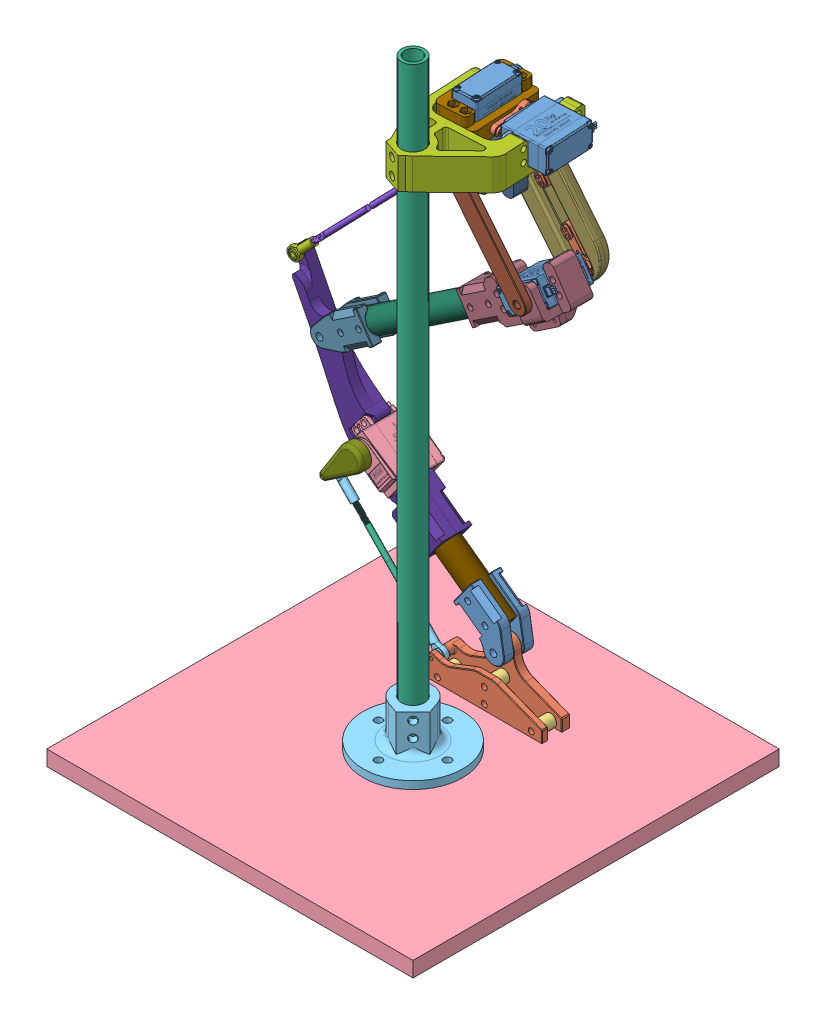
SolidWorks assembly Assembly 1, configuration Default. Lengths in mm.
Overall size (328.16 522.22 516.1).
41 component instances, 25 part files, 59 mates.
Components (placement in the parent):
- Servo_Body^Assembly 1-1: Servo_Body^Assembly 1 [Default] at (148.642 192.4655 -24.1058) x (-0.998744 0 0.050107) z (0.050107 0 0.998744) size (20.1 45.99 55.6) (virtual)
- Servo_Arm^Assembly 1-2: Servo_Arm^Assembly 1 [Default] at (148.642 192.4655 -24.1058) x (0 0 1) z (1 0 0) size (14.5 6.95 35.53) (virtual)
- Servo_Arm^Assembly 1-4: Servo_Arm^Assembly 1 [Default] at (147.142 155.4655 -30.1058) x (0.778746 0.62734 0) z (-0.62734 0.778746 0) size (14.5 6.95 35.53) (virtual)
- Servo_Body^Assembly 1-3: Servo_Body^Assembly 1 [Default] at (147.142 155.4655 -30.1058) x (0 1 0) z (-1 0 0) size (20.1 45.99 55.6) (virtual)
- Servo Arm^Assembly 1-1: Servo Arm^Assembly 1 [Default] at (54.4738 -91.7116 -17.6058) x (-0.717765 0.696286 0) z (0.696286 0.717765 0) size (14.5 6.95 35.53) (virtual)
- Servo Body^Assembly 1-1: Servo Body^Assembly 1 [Default] at (54.4738 -91.7116 -17.6058) x (0.591048 0.806636 0) z (0.806636 -0.591048 0) size (20.1 45.99 55.6) (virtual)
- Servo_Body^Assembly 1-2: Servo_Body^Assembly 1 [Default] at (197.3292 93.1658 -30.1058) x (-0.556075 0.831132 0) z (-0.831132 -0.556075 0) size (20.1 45.99 55.6) (virtual)
- Servo_Arm^Assembly 1-5: Servo_Arm^Assembly 1 [Default] at (185.4452 198.4655 -28.956) x (0 -1 0) z (-0.050107 0 -0.998744) size (14.5 6.95 35.53) (virtual)
- Servo_Body^Assembly 1-4: Servo_Body^Assembly 1 [Default] at (184.4465 198.4655 -28.9059) x (0 1 0) z (0.050107 0 0.998744) size (20.1 45.99 55.6) (virtual)
- Servo_Arm^Assembly 1-3: Servo_Arm^Assembly 1 [Default] at (197.3292 93.1658 -30.1058) x (-0.778746 -0.62734 0) z (0.62734 -0.778746 0) size (14.5 6.95 35.53) (virtual)
- M4 Linkage 2^Assembly 1-2: M4 Linkage 2^Assembly 1 [Default] at (58.3069 -141.5928 -5.5558) x (-0.706028 -0.685079 -0.17942) z (0.69638 -0.717674 0) size (18.79 7.88 136) (virtual)
  - M3 Ball Joint Rod End^M4 Linkage 2_Assembly 1-1: M3 Ball Joint Rod End^M4 Linkage 2_Assembly 1 [59935K14] at (0 0 75) x (-0.983773 0.17942 0) z (0.17942 0.983773 0) size (11 28.3 6) (virtual)
  - M4 Connecting Rod^M4 Linkage 2_Assembly 1-1: M4 Connecting Rod^M4 Linkage 2_Assembly 1 [6516K132] at origin size (4.62 4.16 100.16) (virtual)
  - M3 Ball Joint Rod End^M4 Linkage 2_Assembly 1-2: M3 Ball Joint Rod End^M4 Linkage 2_Assembly 1 [59935K14] at (0 0 -25) x (0.983773 -0.17942 0) z (0.17942 0.983773 0) size (11 28.3 6) (virtual)
- M4 Linkage 1^Assembly 1-3: M4 Linkage 1^Assembly 1 [Default] at (45.9964 73.679 -18.6558) x (-0.70731 0.683755 -0.17942) z (-0.695033 -0.718977 0) size (11.9 7.88 190) (virtual)
  - M3 Ball Joint Rod End^M4 Linkage 1_Assembly 1-1: M3 Ball Joint Rod End^M4 Linkage 1_Assembly 1 [59935K14] at (0 0 75) x (-0.983773 0.17942 0) z (0.17942 0.983773 0) size (11 28.3 6) (virtual)
  - M4 Connecting Rod^M4 Linkage 1_Assembly 1-1: M4 Connecting Rod^M4 Linkage 1_Assembly 1 [6516K132] at origin size (4.62 4.16 154.16) (virtual)
  - M3 Ball Joint Rod End^M4 Linkage 1_Assembly 1-2: M3 Ball Joint Rod End^M4 Linkage 1_Assembly 1 [59935K14] at (0 0 -79) x (0.983773 -0.17942 0) z (0.17942 0.983773 0) size (11 28.3 6) (virtual)
- Hip 1^Assembly 1-3: Hip 1^Assembly 1 [Default] at (149.1431 198.4655 -14.1184) x (0.050107 0 0.998744) z (0.998744 0 -0.050107) size (60 20 32) (virtual)
- Hip 2^Assembly 1-3: Hip 2^Assembly 1 [Default] at (137.142 155.4655 -24.1058) x (1 0 0) z (0 1 0) size (62.55 33.6 37) (virtual)
- Thigh inner^Assembly 1-1: Thigh inner^Assembly 1 [Default] at (147.142 155.4655 6.4942) x (0.62734 -0.778746 0) z (0.778746 0.62734 0) size (95 6 15) (virtual)
- Thigh Outer^Assembly 1-1: Thigh Outer^Assembly 1 [Default] at (147.142 155.4655 -54.1058) x (0.62734 -0.778746 0) z (-0.778746 -0.62734 0) size (101 12.91 45) (virtual)
- Foreleg^Assembly 1-1: Foreleg^Assembly 1 [Default] at (20.1296 -30.1009 -17.6058) x (0.98242 -0.186684 0) z (0 0 1) size (196.97 194.09 159.12) (virtual)
  - Foreleg upper^Foreleg_Assembly 1-2: Foreleg upper^Foreleg_Assembly 1 [Default] at (143.9453 147.1654 -6.5) x (-0.71271 -0.701458 0) z (0.701458 -0.71271 0) size (90 34.23 40) (virtual)
  - Foreleg lower^Foreleg_Assembly 1-1: Foreleg lower^Foreleg_Assembly 1 [Default<As Machined>] at (211.6528 213.804 0) x (-0.593335 -0.804955 0) z (0 0 1) size (54.23 29.24 25) (virtual)
  - Pipe^Foreleg_Assembly 1-1: Pipe^Foreleg_Assembly 1 [Default] at (-15.6593 20.1147 -3.3296) x (0.23303 0.779273 0.581748) z (-0.581748 0.59108 -0.558742) size (127.4 125.81 19.05) (virtual)
- Servo Cover^Assembly 1-1: Servo Cover^Assembly 1 [Default] at (-106.6902 27.004 -15.2721) x (0.996744 0.044176 0.067458) z (-0.072355 0.12072 0.990046) size (37 36.07 11.56) (virtual)
- Shin^Assembly 1-1: Shin^Assembly 1 [Default] at (-9.6004 -3.0399 -16.3225) x (0.995998 0.08937 0) z (0 0 1) size (173.01 220.81 25) (virtual)
  - Shin^Shin_Assembly 1-1: Shin^Shin_Assembly 1 [Default] at (26.0363 -25.7805 -1.2832) size (126.76 169.15 25) (virtual)
  - shin pipe^Shin_Assembly 1-1: shin pipe^Shin_Assembly 1 [Default] at (155.3385 -180.9229 -1.2832) x (0.232016 0.263552 0.936327) z (-0.618699 -0.702794 0.351128) size (19.05 90 19.05) (virtual)
  - Ankle^Shin_Assembly 1-1: Ankle^Shin_Assembly 1 [Default] at (-50.3662 41.4799 -1.2832) size (40.26 50.64 25) (virtual)
- Foot^Assembly 1-1: Foot^Assembly 1 [Default] at (-43.273 53.1793 -17.6058) size (97 46.2 23.5) (virtual)
  - foot^Foot_Assembly 1-1: foot^Foot_Assembly 1 [Default] at (206.6131 -235.2675 0) size (97 46.1 23.5) (virtual)
  - Foot Spacer^Foot_Assembly 1-1: Foot Spacer^Foot_Assembly 1 [Default] at (206.6131 -255.7675 3.5) size (10.2 10.2 11.5) (virtual)
  - Foot Spacer^Foot_Assembly 1-2: Foot Spacer^Foot_Assembly 1 [Default] at (245.6131 -268.2675 3.5) size (10.2 10.2 11.5) (virtual)
  - Foot Spacer^Foot_Assembly 1-3: Foot Spacer^Foot_Assembly 1 [Default] at (167.6131 -268.2675 3.5) size (10.2 10.2 11.5) (virtual)
  - Foot Spacer^Foot_Assembly 1-4: Foot Spacer^Foot_Assembly 1 [Default] at (206.6131 -268.2675 3.5) size (10.2 10.2 11.5) (virtual)
- Wooden Base^Assembly 1-1: Wooden Base^Assembly 1 [Default] at origin size (304.8 12.7 304.8) (virtual)
- Adaptor^Assembly 1-1: Adaptor^Assembly 1 [Default] at origin size (82.85 38.1 82.85) (virtual)
- Test Pipe^Assembly 1-1: Test Pipe^Assembly 1 [Default] at (131.6422 -241.4727 56.997) x (-0.103745 0.71271 0.693744) z (-0.989002 0 -0.147899) size (369.72 364.31 19.05) (virtual)
- Test Bench Adaptor v1^Assembly 1-1: Test Bench Adaptor v1^Assembly 1 [Default] at (190.94 198.4655 -19.2191) x (0.050107 0 0.998744) z (0 -1 0) size (113.75 73 26) (virtual)
Mates (geometry in assembly coordinates):
- Coincident1: coincident anti-aligned: plane of Servo Body^Assembly 1-1 through (54.4738 -91.7116 0.7942) normal (0 0 1); plane of Servo Arm^Assembly 1-1 through (54.4738 -91.7116 0.7942) normal (0 0 -1)
- Concentric1: concentric anti-aligned: cylinder of Servo Arm^Assembly 1-1 through (54.4738 -91.7116 0.7942) axis (0 0 -1) radius 2.5; cylinder of Servo Body^Assembly 1-1 through (54.4738 -91.7116 -4.1058) axis (0 0 1) radius 3.8
- Concentric15: concentric aligned: cylinder of Servo Body^Assembly 1-1 through (84.8547 -107.774 -23.9698) axis (0 0 1) radius 2.25; cylinder of Shin^Assembly 1-1/Shin^Shin_Assembly 1-1 through (84.8547 -107.774 -30.1058) axis (0 0 1) radius 2.1
- Concentric16: concentric aligned: cylinder of Servo Body^Assembly 1-1 through (78.9442 -115.8404 -23.9698) axis (0 0 1) radius 2.25; cylinder of Shin^Assembly 1-1/Shin^Shin_Assembly 1-1 through (78.9442 -115.8404 -30.1058) axis (0 0 1) radius 2.1
- Coincident10: coincident anti-aligned: plane of Servo Body^Assembly 1-1 through (81.5725 -100.4102 -17.6058) normal (0 0 -1); plane of Shin^Assembly 1-1/Shin^Shin_Assembly 1-1 through (93.3552 -103.4651 -17.6058) normal (0 0 1)
- Width5: width anti-aligned: plane of Foot^Assembly 1-1/foot^Foot_Assembly 1-1 through (119.2402 -204.3893 -14.1058) normal (0 0 1); plane of Shin^Assembly 1-1/Ankle^Shin_Assembly 1-1 through (119.2402 -204.3893 -21.1058) normal (0 0 -1); plane of Foot^Assembly 1-1/foot^Foot_Assembly 1-1 through (164.0486 -202.3736 -13.6058) normal (0 0 -1); plane of Shin^Assembly 1-1/Ankle^Shin_Assembly 1-1 through (164.0486 -202.3736 -21.6058) normal (0 0 1)
- Concentric5: concentric anti-aligned: cylinder of Servo_Arm^Assembly 1-2 through (148.642 174.0655 -24.1058) axis (0 1 0) radius 2.5; cylinder of Servo_Body^Assembly 1-1 through (148.642 178.9655 -24.1058) axis (0 -1 0) radius 3.8
- Coincident5: coincident anti-aligned: plane of Servo_Body^Assembly 1-1 through (148.642 174.0655 -24.1058) normal (0 -1 0); plane of Servo_Arm^Assembly 1-2 through (148.642 174.0655 -24.1058) normal (0 1 0)
- Concentric20: concentric anti-aligned: circle of Servo_Arm^Assembly 1-2; cylinder of Hip 2^Assembly 1-3 through (124.142 139.4655 -24.1058) axis (0 1 0) radius 1.45
- Concentric21: concentric anti-aligned: circle of Servo_Arm^Assembly 1-2; cylinder of Hip 2^Assembly 1-3 through (148.642 139.4655 -24.1058) axis (0 1 0) radius 1.45
- Coincident11: coincident anti-aligned: plane of Servo_Arm^Assembly 1-2 through (138.292 171.4655 -10.3058) normal (0 -1 0); plane of Hip 2^Assembly 1-3 through (137.142 171.4655 -30.1058) normal (0 1 0)
- Concentric22: concentric anti-aligned: cylinder of Servo_Body^Assembly 1-2 through (197.3292 93.1658 -43.6058) axis (0 0 -1) radius 3.8; cylinder of Servo_Arm^Assembly 1-3 through (197.3292 93.1658 -48.5058) axis (0 0 1) radius 2.5
- Coincident12: coincident anti-aligned: plane of Servo_Body^Assembly 1-2 through (197.3292 93.1658 -48.5058) normal (0 0 -1); plane of Servo_Arm^Assembly 1-3 through (197.3292 93.1658 -48.5058) normal (0 0 1)
- Concentric35: concentric anti-aligned: cylinder of Servo_Arm^Assembly 1-4 through (147.142 155.4655 -48.5058) axis (0 0 1) radius 2.5; cylinder of Servo_Body^Assembly 1-3 through (147.142 155.4655 -43.6058) axis (0 0 -1) radius 3.8
- Coincident25: coincident anti-aligned: plane of Servo_Arm^Assembly 1-4 through (147.142 155.4655 -48.5058) normal (0 0 1); plane of Servo_Body^Assembly 1-3 through (147.142 155.4655 -48.5058) normal (0 0 -1)
- Concentric36: concentric aligned: circle of Servo_Body^Assembly 1-3; cylinder of Hip 2^Assembly 1-3 through (113.142 160.4655 -18.1058) axis (0 0 -1) radius 2.4
- Concentric37: concentric aligned: circle of Servo_Body^Assembly 1-3; cylinder of Hip 2^Assembly 1-3 through (161.142 160.4655 -18.1058) axis (0 0 -1) radius 2.4
- Coincident26: coincident anti-aligned: plane of Servo_Body^Assembly 1-3 through (120.142 164.4655 -30.1058) normal (0 0 1); plane of Hip 2^Assembly 1-3 through (137.142 155.4655 -30.1058) normal (0 0 -1)
- Coincident27: coincident anti-aligned: plane of Servo_Body^Assembly 1-2 through (169.8839 85.632 -30.1058) normal (0 0 1); plane of Foreleg^Assembly 1-1/Foreleg upper^Foreleg_Assembly 1-2 through (189.0179 87.605 -30.1058) normal (0 0 -1)
- Concentric50: concentric anti-aligned: cylinder of Shin^Assembly 1-1/Shin^Shin_Assembly 1-1 through (18.6358 -26.3903 -5.1058) axis (0 0 -1) radius 3.1; cylinder of Foreleg^Assembly 1-1/Foreleg lower^Foreleg_Assembly 1-1 through (18.6358 -26.3903 -30.1058) axis (0 0 1) radius 2.9
- Width7: width anti-aligned: plane of Foreleg^Assembly 1-1/Foreleg lower^Foreleg_Assembly 1-1 through (18.6358 -26.3903 -5.1058) normal (0 0 1); plane of Foreleg^Assembly 1-1/Foreleg lower^Foreleg_Assembly 1-1 through (18.6358 -26.3903 -30.1058) normal (0 0 -1); plane of Shin^Assembly 1-1/Shin^Shin_Assembly 1-1 through (18.6358 -26.3903 -21.6058) normal (0 0 -1); plane of Shin^Assembly 1-1/Shin^Shin_Assembly 1-1 through (18.6358 -26.3903 -13.6058) normal (0 0 1)
- Concentric53: concentric anti-aligned: cylinder of Servo_Body^Assembly 1-2 through (206.1846 105.1065 -23.7418) axis (0 0 -1) radius 2.25; cylinder of Foreleg^Assembly 1-1/Foreleg upper^Foreleg_Assembly 1-2 through (206.1846 105.1065 -30.1058) axis (0 0 1) radius 2.45
- Concentric54: concentric anti-aligned: cylinder of Servo_Body^Assembly 1-2 through (211.7454 96.7952 -23.7418) axis (0 0 -1) radius 2.25; cylinder of Foreleg^Assembly 1-1/Foreleg upper^Foreleg_Assembly 1-2 through (211.7454 96.7952 -30.1058) axis (0 0 1) radius 2.45
- Delete later: parallel: line of Hip 2^Assembly 1-3 through (157.192 167.4655 3.4942) axis (-1 0 0)
- Origin mate: coordinate: point of Foot^Assembly 1-1
- Concentric76: concentric anti-aligned: cylinder of M4 Linkage 2^Assembly 1-2/M3 Ball Joint Rod End^M4 Linkage 2_Assembly 1-2 through (32.1927 -114.6801 -2.5558) axis (0 0 -1) radius 2; cylinder of Servo Cover^Assembly 1-1 through (32.1927 -114.6801 -2.6058) axis (0 0 1) radius 1.4
- Concentric77: concentric aligned: cylinder of Servo Arm^Assembly 1-1 through (54.4738 -91.7116 -2.6058) axis (0 0 1) radius 7.25; cylinder of Servo Cover^Assembly 1-1 through (54.4738 -91.7116 -2.6058) axis (0 0 1) radius 7.55
- Concentric78: concentric aligned: circle of Servo Arm^Assembly 1-1; cylinder of Servo Cover^Assembly 1-1 through (37.4148 -109.2968 -2.6058) axis (0 0 1) radius 4.1
- Coincident43: coincident anti-aligned: plane of Servo Arm^Assembly 1-1 through (37.3621 -89.5317 3.3942) normal (0 0 1); plane of Servo Cover^Assembly 1-1 through (37.4148 -109.2968 3.3942) normal (0 0 -1)
- Concentric82: concentric aligned: cylinder of M4 Linkage 2^Assembly 1-2/M3 Ball Joint Rod End^M4 Linkage 2_Assembly 1-1 through (119.2402 -204.3893 -2.5558) axis (0 0 -1) radius 2; cylinder of Foot^Assembly 1-1/foot^Foot_Assembly 1-1 through (119.2402 -204.3893 2.3942) axis (0 0 -1) radius 1.4
- Concentric83: concentric aligned: cylinder of M4 Linkage 1^Assembly 1-3/M3 Ball Joint Rod End^M4 Linkage 1_Assembly 1-2 through (109.592 139.4655 -15.6558) axis (0 0 -1) radius 2; cylinder of Hip 2^Assembly 1-3 through (109.592 139.4655 3.4942) axis (0 0 -1) radius 1.4
- Concentric84: concentric aligned: cylinder of M4 Linkage 1^Assembly 1-3/M3 Ball Joint Rod End^M4 Linkage 1_Assembly 1-1 through (-14.819 10.7685 -15.6558) axis (0 0 -1) radius 2; cylinder of Shin^Assembly 1-1/Shin^Shin_Assembly 1-1 through (-14.819 10.7685 -5.1058) axis (0 0 -1) radius 1.4
- Distance1: distance = 0.5 mm anti-aligned: plane of M4 Linkage 2^Assembly 1-2/M3 Ball Joint Rod End^M4 Linkage 2_Assembly 1-2 through (32.3098 -106.9028 -3.1058) normal (0 0 1); plane of Servo Cover^Assembly 1-1 through (32.1927 -114.6801 -2.6058) normal (0 0 -1)
- Concentric86: concentric aligned: cylinder of Thigh inner^Assembly 1-1 through (197.3292 93.1658 3.4942) axis (0 0 1) radius 2.6; cylinder of Foreleg^Assembly 1-1/Foreleg upper^Foreleg_Assembly 1-2 through (197.3292 93.1658 -6.5058) axis (0 0 1) radius 2.4
- Concentric2: concentric aligned: cylinder of Thigh inner^Assembly 1-1 through (147.142 155.4655 3.4942) axis (0 0 1) radius 2.6; cylinder of Hip 2^Assembly 1-3 through (147.142 155.4655 -6.5058) axis (0 0 1) radius 2.4
- Concentric87: concentric aligned: circle of Servo_Arm^Assembly 1-3; cylinder of Thigh Outer^Assembly 1-1 through (181.9594 112.2451 -51.1058) axis (0 0 -1) radius 1.4
- Coincident44: coincident anti-aligned: plane of Servo_Arm^Assembly 1-3 through (180.0895 92.5685 -51.1058) normal (0 0 -1); plane of Thigh Outer^Assembly 1-1 through (147.142 155.4655 -51.1058) normal (0 0 1)
- Coincident45: coincident anti-aligned: plane of Servo_Arm^Assembly 1-4 through (164.3817 156.0627 -51.1058) normal (0 0 -1); plane of Thigh Outer^Assembly 1-1 through (147.142 155.4655 -51.1058) normal (0 0 1)
- Concentric88: concentric aligned: circle of Servo_Arm^Assembly 1-4; cylinder of Thigh Outer^Assembly 1-1 through (162.5118 136.3862 -51.1058) axis (0 0 -1) radius 1.4
- Concentric89: concentric aligned: cylinder of Servo_Arm^Assembly 1-3 through (197.3292 93.1658 -50.1058) axis (0 0 -1) radius 3.85; cylinder of Thigh Outer^Assembly 1-1 through (197.3292 93.1658 -45.1058) axis (0 0 -1) radius 1.4
- Concentric90: concentric aligned: cylinder of Servo_Arm^Assembly 1-4 through (147.142 155.4655 -45.1058) axis (0 0 -1) radius 7.25; cylinder of Thigh Outer^Assembly 1-1 through (147.142 155.4655 -45.1058) axis (0 0 -1) radius 1.4
- Coincident46: coincident anti-aligned: plane of Foreleg^Assembly 1-1/Foreleg upper^Foreleg_Assembly 1-2 through (233.1416 117.1264 3.4942) normal (0 0 1); plane of Thigh inner^Assembly 1-1 through (147.142 155.4655 3.4942) normal (0 0 -1)
- Concentric91: concentric aligned: cylinder of Servo_Body^Assembly 1-1 through (142.9468 198.8294 -37.8377) axis (0 -1 0) radius 2.25; cylinder of Hip 1^Assembly 1-3 through (142.9468 204.4655 -37.8377) axis (0 -1 0) radius 2.4
- Concentric92: concentric aligned: cylinder of Servo_Body^Assembly 1-1 through (152.9342 198.8294 -38.3387) axis (0 -1 0) radius 2.25; cylinder of Hip 1^Assembly 1-3 through (152.9342 204.4655 -38.3387) axis (0 -1 0) radius 2.4
- Coincident47: coincident anti-aligned: plane of Servo_Body^Assembly 1-1 through (141.0062 192.4655 3.3113) normal (0 1 0); plane of Hip 1^Assembly 1-3 through (149.1431 192.4655 -14.1184) normal (0 -1 0)
- Concentric93: concentric anti-aligned: circle of Servo_Arm^Assembly 1-5; circle of Hip 1^Assembly 1-1
- Concentric94: concentric aligned: cylinder of Servo_Arm^Assembly 1-5 through (167.0683 198.4655 -28.034) axis (0.998744 0 -0.050107) radius 2.5; cylinder of Hip 1^Assembly 1-3 through (132.5118 198.4655 -26.3003) axis (0.998744 0 -0.050107) radius 1.45
- Concentric95: concentric anti-aligned: cylinder of Servo_Arm^Assembly 1-5 through (167.0683 198.4655 -28.034) axis (0.998744 0 -0.050107) radius 2.5; cylinder of Servo_Body^Assembly 1-4 through (170.0645 198.4655 -28.1843) axis (-0.998744 0 0.050107) radius 1.25
- Coincident48: coincident anti-aligned: plane of Servo_Arm^Assembly 1-5 through (170.9826 184.6655 -17.8674) normal (0.998744 0 -0.050107); plane of Servo_Body^Assembly 1-4 through (170.464 198.4655 -28.2044) normal (-0.998744 0 0.050107)
- Coincident49: coincident anti-aligned: plane of Servo_Arm^Assembly 1-5 through (164.9902 184.6655 -17.5667) normal (-0.998744 0 0.050107); plane of Hip 1^Assembly 1-3 through (165.123 192.4655 -14.9201) normal (0.998744 0 -0.050107)
- Concentric96: concentric aligned: cylinder of Adaptor^Assembly 1-1 through (152.4 -190.5 50.8) axis (0 -1 0) radius 9.675; cylinder of Test Pipe^Assembly 1-1 through (152.4 271.4 50.8) axis (0 -1 0) radius 9.525
- Coincident50: coincident aligned: plane of Wooden Base^Assembly 1-1 through (0 -228.6 0) normal (0 1 0); circle of Test Pipe^Assembly 1-1
- Distance2: distance = 0.5 mm anti-aligned: plane of M4 Linkage 1^Assembly 1-3/M3 Ball Joint Rod End^M4 Linkage 1_Assembly 1-2 through (117.3691 139.5971 -21.1058) normal (0 0 -1); plane of Hip 2^Assembly 1-3 through (137.142 155.4655 -21.6058) normal (0 0 1)
- Concentric97: concentric anti-aligned: circle of Servo_Body^Assembly 1-4; cylinder of Test Bench Adaptor v1^Assembly 1-1 through (198.135 203.4655 4.4501) axis (-0.998744 0 0.050107) radius 2.4
- Concentric98: concentric aligned: cylinder of Servo_Body^Assembly 1-4 through (192.5061 193.4655 4.7326) axis (-0.998744 0 0.050107) radius 2.25; cylinder of Test Bench Adaptor v1^Assembly 1-1 through (198.135 193.4655 4.4501) axis (-0.998744 0 0.050107) radius 2.4
- Coincident53: coincident anti-aligned: plane of Servo_Body^Assembly 1-4 through (185.7993 207.4655 -1.9398) normal (0.998744 0 -0.050107); plane of Test Bench Adaptor v1^Assembly 1-1 through (186.7875 300.3038 17.7571) normal (-0.998744 0 0.050107)
- Concentric99: concentric aligned: cylinder of Test Pipe^Assembly 1-1 through (152.4 271.4 50.8) axis (0 -1 0) radius 9.525; cylinder of Test Bench Adaptor v1^Assembly 1-1 through (152.4 300.3038 50.8) axis (0 -1 0) radius 9.725
- Concentric100: concentric aligned: cylinder of Shin^Assembly 1-1/Ankle^Shin_Assembly 1-1 through (163.3402 -182.0882 -5.1058) axis (0 0 -1) radius 2.9; cylinder of Foot^Assembly 1-1/foot^Foot_Assembly 1-1 through (163.3402 -182.0882 -14.1058) axis (0 0 -1) radius 3.1
- Parallel3: parallel: line of Foot^Assembly 1-1/foot^Foot_Assembly 1-1 through (210.8402 -219.5882 -21.1058) axis (-1 0 0); plane of Wooden Base^Assembly 1-1 through (0 -228.6 0) normal (0 1 0)
